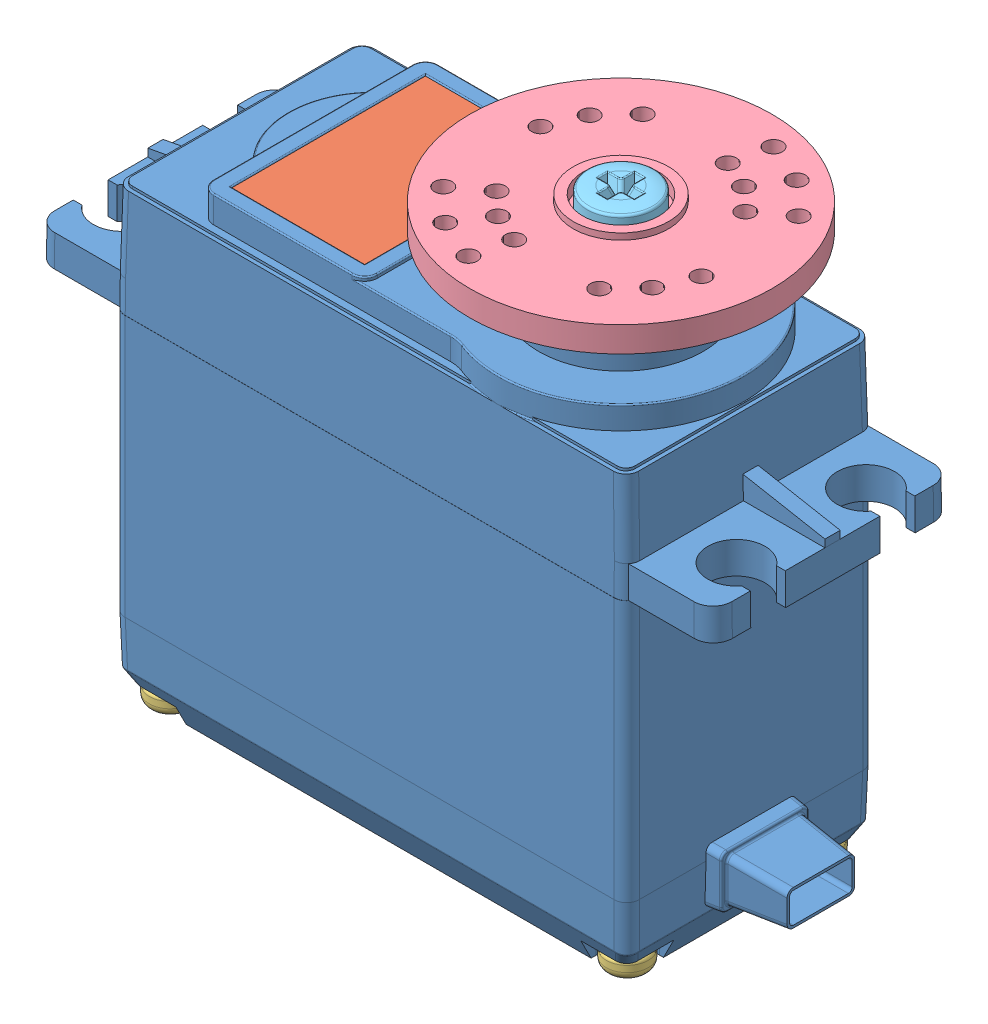
SolidWorks assembly ROBOT SERVO Hitec HSR-2645CR СБ, configuration По умолчанию. Lengths in mm.
Overall size (53.4 45.61 32.94).
8 component instances, 5 part files, 15 mates.
Components (placement in the parent):
- ROBOT SERVO Hitec HSR-2645CR-1: ROBOT SERVO Hitec HSR-2645CR [По умолчанию] at origin size (53.4 42.9 19.6)
- Наклейка сервы-1: Наклейка сервы [По умолчанию] at (-7.8411 37.7 -0.0485) x (0.009787 0 -0.999952) z (0.999952 0 0.009787) size (15.38 0.01 10.64)
- ROBOT SERVO Hitec HSR-2645CR винт-1: ROBOT SERVO Hitec HSR-2645CR винт [По умолчанию] at (18 34.1 7.5) x (-0.614203 0 -0.789148) z (-0.789148 0 0.614203) size (3.3 34.05 3.3)
- ROBOT SERVO Hitec HSR-2645CR винт-2: ROBOT SERVO Hitec HSR-2645CR винт [По умолчанию] at (18 34.1 -7.5) x (-0.614203 0 -0.789148) z (-0.789148 0 0.614203) size (3.3 34.05 3.3)
- ROBOT SERVO Hitec HSR-2645CR винт-3: ROBOT SERVO Hitec HSR-2645CR винт [По умолчанию] at (-18 34.1 7.5) x (-0.614203 0 -0.789148) z (-0.789148 0 0.614203) size (3.3 34.05 3.3)
- ROBOT SERVO Hitec HSR-2645CR винт-4: ROBOT SERVO Hitec HSR-2645CR винт [По умолчанию] at (-18 34.1 -7.5) x (-0.227126 0 -0.973865) z (-0.973865 0 0.227126) size (3.3 34.05 3.3)
- ROBOT SERVO Hitec HSR-2645CR фланец-1: ROBOT SERVO Hitec HSR-2645CR фланец [По умолчанию] at (10 44.5 0) x (-0.837169 0 -0.546944) z (-0.546944 0 0.837169) size (23.8 5 23.8)
- ROBOT SERVO Hitec HSR-2645CR винт 2-1: ROBOT SERVO Hitec HSR-2645CR винт 2 [По умолчанию] at (10 36.5 0) size (5.3 9.11 5.3)
Mates (geometry in assembly coordinates):
- Совпадение1: coincident anti-aligned: plane of ROBOT SERVO Hitec HSR-2645CR-1 through (0 37.7 0) normal (0 1 0); plane of Наклейка сервы-1 through (-7.8411 37.7 -0.0485) normal (0 -1 0)
- Ширина1: width aligned: plane of Наклейка сервы-1 through (-2.5556 37.7 7.6394) normal (0 0 1); plane of Наклейка сервы-1 through (-13.0444 37.7 -7.6394) normal (0 0 -1); plane of ROBOT SERVO Hitec HSR-2645CR-1 through (6.0163 34.7 8.84) normal (0 0 1); plane of ROBOT SERVO Hitec HSR-2645CR-1 through (6.0163 34.7 -8.84) normal (0 0 -1)
- Ширина2: width anti-aligned: plane of Наклейка сервы-1 through (-2.5556 37.7 -7.7394) normal (1 0 0); plane of Наклейка сервы-1 through (-13.0444 37.7 7.6394) normal (-1 0 0); plane of ROBOT SERVO Hitec HSR-2645CR-1 through (-14.25 34.7 8.84) normal (-1 0 0); plane of ROBOT SERVO Hitec HSR-2645CR-1 through (-1.35 37.8 -8.84) normal (1 0 0)
- Концентричный1: concentric anti-aligned: cylinder of ROBOT SERVO Hitec HSR-2645CR-1 through (-18 11.6 -7.5) axis (0 -1 0) radius 0.9; cylinder of ROBOT SERVO Hitec HSR-2645CR винт-4 through (-18 0.1 -7.5) axis (0 1 0) radius 0.8
- Концентричный2: concentric anti-aligned: cylinder of ROBOT SERVO Hitec HSR-2645CR-1 through (-18 11.6 7.5) axis (0 -1 0) radius 0.9; cylinder of ROBOT SERVO Hitec HSR-2645CR винт-3 through (-18 0.1 7.5) axis (0 1 0) radius 0.8
- Концентричный3: concentric anti-aligned: cylinder of ROBOT SERVO Hitec HSR-2645CR-1 through (18 11.6 7.5) axis (0 -1 0) radius 0.9; cylinder of ROBOT SERVO Hitec HSR-2645CR винт-1 through (18 0.1 7.5) axis (0 1 0) radius 0.8
- Концентричный4: concentric anti-aligned: cylinder of ROBOT SERVO Hitec HSR-2645CR-1 through (18 11.6 -7.5) axis (0 -1 0) radius 0.9; cylinder of ROBOT SERVO Hitec HSR-2645CR винт-2 through (18 0.1 -7.5) axis (0 1 0) radius 0.8
- Совпадение2: coincident anti-aligned: plane of ROBOT SERVO Hitec HSR-2645CR-1 through (0 1.6 0) normal (0 -1 0); plane of ROBOT SERVO Hitec HSR-2645CR винт-4 through (-18 1.6 -7.5) normal (0 1 0)
- Совпадение3: coincident anti-aligned: plane of ROBOT SERVO Hitec HSR-2645CR-1 through (0 1.6 0) normal (0 -1 0); plane of ROBOT SERVO Hitec HSR-2645CR винт-3 through (-18 1.6 7.5) normal (0 1 0)
- Совпадение4: coincident anti-aligned: plane of ROBOT SERVO Hitec HSR-2645CR-1 through (0 1.6 0) normal (0 -1 0); plane of ROBOT SERVO Hitec HSR-2645CR винт-1 through (18 1.6 7.5) normal (0 1 0)
- Совпадение5: coincident anti-aligned: plane of ROBOT SERVO Hitec HSR-2645CR-1 through (0 1.6 0) normal (0 -1 0); plane of ROBOT SERVO Hitec HSR-2645CR винт-2 through (18 1.6 -7.5) normal (0 1 0)
- Концентричный6: concentric anti-aligned: cylinder of ROBOT SERVO Hitec HSR-2645CR-1 through (10 39.65 0) axis (0 -1 0) radius 6.475; cylinder of ROBOT SERVO Hitec HSR-2645CR фланец-1 through (10 40 0) axis (0 1 0) radius 4.45
- Расстояние1: distance = 44.5 mm anti-aligned: plane of ROBOT SERVO Hitec HSR-2645CR фланец-1 through (10 44.5 0) normal (0 1 0); plane of ROBOT SERVO Hitec HSR-2645CR-1 through (0 0 0) normal (0 -1 0)
- Концентричный7: concentric anti-aligned: cylinder of ROBOT SERVO Hitec HSR-2645CR-1 through (10 42.9 0) axis (0 1 0) radius 1.025; cylinder of ROBOT SERVO Hitec HSR-2645CR винт 2-1 through (10 48.865 0) axis (0 -1 0) radius 1.25
- Совпадение6: coincident anti-aligned: plane of ROBOT SERVO Hitec HSR-2645CR фланец-1 through (10 44 0) normal (0 1 0); plane of ROBOT SERVO Hitec HSR-2645CR винт 2-1 through (10 44 0) normal (0 -1 0)
